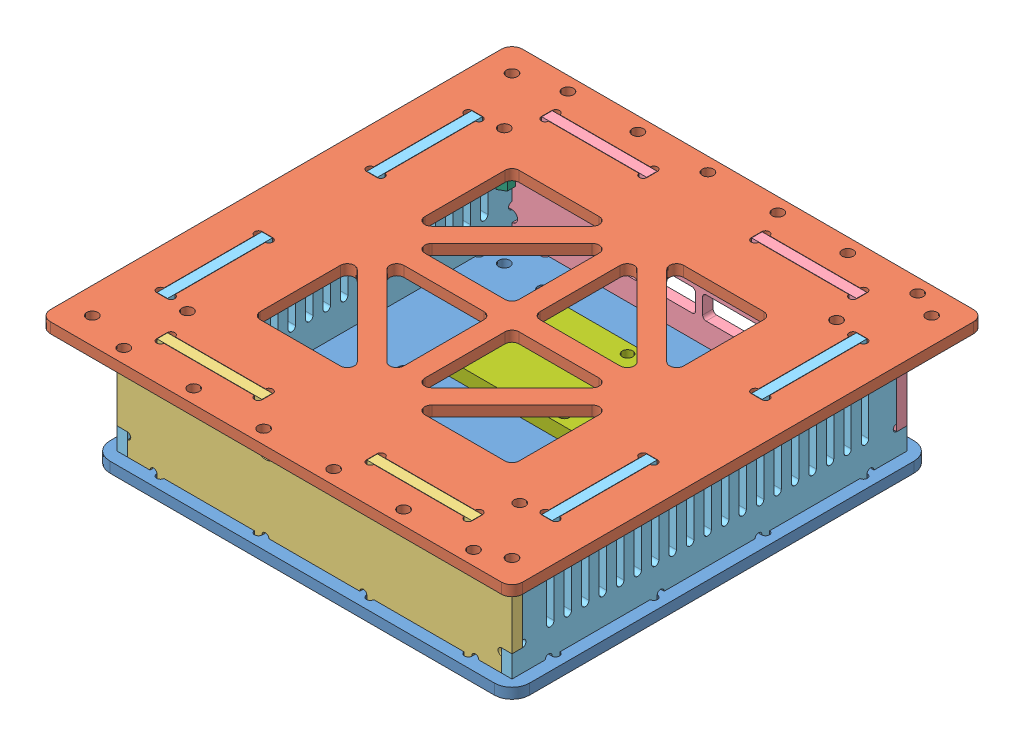
SolidWorks assembly 王八壳, configuration Default. Lengths in mm.
Overall size (135 50.48 135).
13 component instances, 9 part files, 35 mates.
Components (placement in the parent):
- 王八底壳-1: 王八底壳 [Default] at (0 52.2554 0) size (120 3 120)
- 王八顶壳-1: 王八顶壳 [Default] at (0 85.7554 0) size (135 3 135)
- 王八1-1: 王八1 [Default] at (0 70.4554 55) x (-1 0 0) z (0 -1 0) size (113 3 36.5)
- 王八3-1: 王八3 [Default] at (0 86.8554 -55) x (-1 0 0) z (0 1 0) size (113 3.1 36.5)
- 王八4-1: 王八4 [Default] at (-55 77.8554 0) x (0 0 -1) z (0 1 0) size (113 3 36.5)
- 王八4-2: 王八4 [Default] at (55 77.8554 0) x (0 0 1) z (0 1 0) size (113 3 36.5)
- 11mm-1: 11mm [Default] at (47.5 74.7554 -45.3) size (4 11 4.62)
- 11mm-2: 11mm [Default] at (47.5 74.7554 45.3) x (0.1665 0 0.986041) z (-0.986041 0 0.1665) size (4 11 4.62)
- 11mm-3: 11mm [Default] at (-47.5 74.7554 -45.3) size (4 11 4.62)
- 11mm-4: 11mm [Default] at (-47.5 74.7554 45.3) size (4 11 4.62)
- NUC5i7RYB-4: NUC5i7RYB [默认] at (0 73.1554 -1.6) (suppressed, hidden)
- 风扇-1: 风扇 [Default] at (-0.5 44.2754 -39.5) size (60 18 30)
- 风扇上壳-1: 风扇上壳 [Default] at (-0.5 26.2754 -39.5) size (80 3 50)
Mates (geometry in assembly coordinates):
- 同心1: concentric aligned: cylinder of 王八底壳-1 through (-47.5 55.2554 45.3) axis (0 -1 0) radius 1.6; cylinder of 王八顶壳-1 through (-47.5 88.7554 45.3) axis (0 -1 0) radius 1.6
- 同心2: concentric aligned: cylinder of 王八底壳-1 through (-47.5 55.2554 -45.3) axis (0 -1 0) radius 1.6; cylinder of 王八顶壳-1 through (-47.5 88.7554 -45.3) axis (0 -1 0) radius 1.6
- 同心5: concentric anti-aligned: circle of 王八顶壳-1; cylinder of 11mm-3 through (-47.5 85.7554 -45.3) axis (0 -1 0) radius 1.5
- 同心6: concentric aligned: cylinder of 王八顶壳-1 through (-47.5 88.7554 45.3) axis (0 -1 0) radius 1.6; cylinder of 11mm-4 through (-47.5 85.7554 45.3) axis (0 -1 0) radius 1.5
- 同心7: concentric aligned: circle of 王八顶壳-1; circle of 11mm-1
- 同心8: concentric aligned: circle of 王八顶壳-1; circle of 11mm-2
- 重合3: coincident anti-aligned: plane of 王八顶壳-1 through (0 85.7554 0) normal (0 -1 0); plane of 11mm-2 through (47.5 85.7554 45.3) normal (0 1 0)
- 重合4: coincident anti-aligned: plane of 王八顶壳-1 through (0 85.7554 0) normal (0 -1 0); plane of 11mm-4 through (-47.5 85.7554 45.3) normal (0 1 0)
- 重合5: coincident anti-aligned: plane of 王八顶壳-1 through (0 85.7554 0) normal (0 -1 0); plane of 11mm-1 through (47.5 85.7554 -45.3) normal (0 1 0)
- 重合6: coincident anti-aligned: plane of 王八顶壳-1 through (0 85.7554 0) normal (0 -1 0); plane of 11mm-3 through (-47.5 85.7554 -45.3) normal (0 1 0)
- 同心9: concentric aligned: circle of 11mm-4; cylinder of NUC5i7RYB-4 through (-47.5 73.1554 45.3) axis (0 1 0) radius 2
- 同心10: concentric anti-aligned: cylinder of 11mm-2 through (47.5 85.7554 45.3) axis (0 -1 0) radius 1.5; cylinder of NUC5i7RYB-4 through (47.5 73.1554 45.3) axis (0 1 0) radius 2
- 重合7: coincident anti-aligned: plane of 11mm-1 through (47.5 74.7554 -45.3) normal (0 -1 0); plane of NUC5i7RYB-4 through (0 74.7554 -1.6) normal (0 1 0)
- 对称1: symmetric aligned: plane of 王八顶壳-1 through (45.1 78.7554 53.4) normal (0 0 1); plane of 王八顶壳-1 through (45.1 78.7554 56.6) normal (0 0 -1); plane of 王八1-1 through (0 70.4554 55) normal (0 0 -1)
- 重合8: coincident anti-aligned: plane of 王八顶壳-1 through (0 85.7554 0) normal (0 -1 0); plane of 王八1-1 through (49.5 85.7554 46.5) normal (0 1 0)
- 对称2: symmetric aligned: plane of 王八顶壳-1 through (-45.1 78.7554 -53.4) normal (0 0 -1); plane of 王八顶壳-1 through (-45.1 78.7554 -56.6) normal (0 0 1); plane of 王八3-1 through (0 86.8554 -55) normal (0 0 1)
- 重合9: coincident anti-aligned: plane of 王八顶壳-1 through (0 85.7554 0) normal (0 -1 0); plane of 王八3-1 through (49.5 85.7554 -46.5) normal (0 1 0)
- 对称3: symmetric aligned: plane of 王八顶壳-1 through (-53.4 78.7554 45.1) normal (-1 0 0); plane of 王八顶壳-1 through (-56.6 78.7554 45.1) normal (1 0 0); plane of 王八4-1 through (-55 77.8554 0) normal (-1 0 0)
- 重合10: coincident anti-aligned: plane of 王八顶壳-1 through (0 85.7554 0) normal (0 -1 0); plane of 王八4-1 through (-46.5 85.7554 47.5) normal (0 1 0)
- 对称4: symmetric aligned: plane of 王八顶壳-1 through (53.4 78.7554 -45.1) normal (1 0 0); plane of 王八顶壳-1 through (56.6 78.7554 -45.1) normal (-1 0 0); plane of 王八4-2 through (55 77.8554 0) normal (1 0 0)
- 重合11: coincident anti-aligned: plane of 王八顶壳-1 through (0 85.7554 0) normal (0 -1 0); plane of 王八4-2 through (46.5 85.7554 -47.5) normal (0 1 0)
- 宽度1: width anti-aligned: plane of 王八顶壳-1 through (-67.5 88.7554 -67.5) normal (0 0 -1); plane of 王八顶壳-1 through (-67.5 88.7554 67.5) normal (0 0 1); plane of 王八4-2 through (21.6998 77.8554 56.5) normal (0 0 1); plane of 王八4-2 through (21.6998 77.8554 -56.5) normal (0 0 -1)
- 宽度2: width anti-aligned: plane of 王八3-1 through (56.5 86.8554 -56.5) normal (1 0 0); plane of 王八3-1 through (-56.5 86.8554 -56.5) normal (-1 0 0); plane of 王八顶壳-1 through (-67.5 88.7554 -67.5) normal (-1 0 0); plane of 王八顶壳-1 through (67.5 88.7554 -67.5) normal (1 0 0)
- 重合12: coincident aligned: plane of 王八1-1 through (56.5 70.4554 87.793) normal (1 0 0); plane of 王八3-1 through (56.5 86.8554 -56.5) normal (1 0 0)
- 重合13: coincident aligned: plane of 王八4-1 through (-21.6998 77.8554 56.5) normal (0 0 1); plane of 王八4-2 through (21.6998 77.8554 56.5) normal (0 0 1)
- 重合14: coincident anti-aligned: plane of 王八底壳-1 through (0 55.2554 0) normal (0 1 0); plane of 王八1-1 through (49.5 55.2554 53.5) normal (0 -1 0)
- 重合15: coincident anti-aligned: plane of 11mm-4 through (-47.5 74.7554 45.3) normal (0 -1 0); plane of NUC5i7RYB-4 through (0 74.7554 -1.6) normal (0 1 0)
- 同心11: concentric anti-aligned: cylinder of 11mm-4 through (-47.5 85.7554 45.3) axis (0 -1 0) radius 1.5; cylinder of NUC5i7RYB-4 through (-47.5 73.1554 45.3) axis (0 1 0) radius 2
- 同心14: concentric anti-aligned: cylinder of 11mm-2 through (47.5 85.7554 45.3) axis (0 -1 0) radius 1.5; cylinder of NUC5i7RYB-4 through (47.5 73.1554 45.3) axis (0 1 0) radius 2
- 重合16: coincident anti-aligned: plane of 王八底壳-1 through (-30.5 62.2554 -40.5) normal (1 0 0); plane of 风扇-1 through (-30.5 29.2754 -9.5) normal (-1 0 0)
- 重合17: coincident anti-aligned: plane of 王八底壳-1 through (-30.5 62.2554 -9.5) normal (0 0 -1); plane of 风扇-1 through (-0.5 44.2754 -9.5) normal (0 0 1)
- 重合18: coincident anti-aligned: plane of NUC5i7RYB-4 through (-1.0006 59.2754 -35.3) normal (0 -1 0); plane of 风扇-1 through (-30.5 59.2754 -9.5) normal (0 1 0)
- 同心15: concentric aligned: cylinder of 风扇-1 through (-27.5208 41.2754 -12.4792) axis (0 1 0) radius 1.5; circle of 风扇上壳-1
- 同心16: concentric aligned: cylinder of 风扇-1 through (-3.4792 41.2754 -12.4792) axis (0 1 0) radius 1.5; circle of 风扇上壳-1
- 重合19: coincident anti-aligned: plane of 风扇-1 through (-0.5 41.2754 -39.5) normal (0 -1 0); plane of 风扇上壳-1 through (-30.5 41.2754 -9.5) normal (0 1 0)
